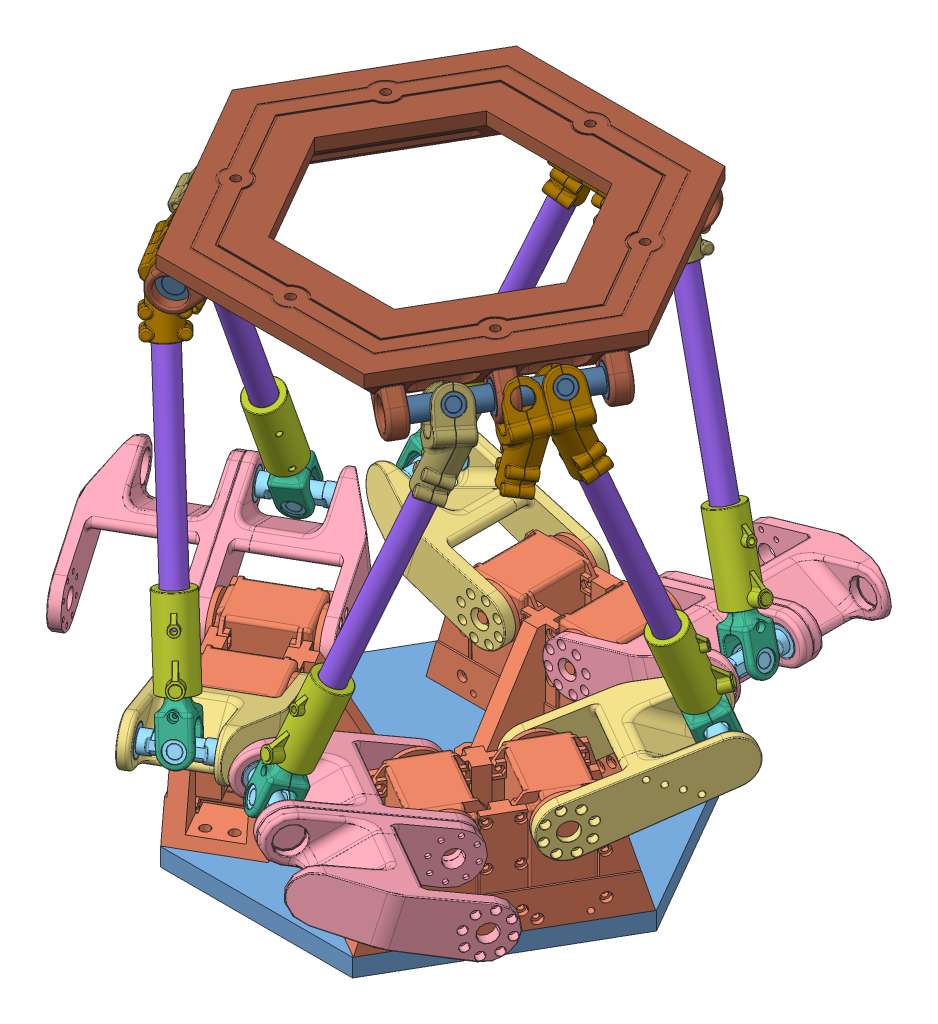
SolidWorks assembly top, configuration Default. Lengths in mm.
Overall size (300.14 294.24 310.35).
47 component instances, 12 part files, 111 mates.
Components (placement in the parent):
- bunn-1: bunn [Default] at origin size (232.33 10 201.21)
- d64hjorne-1: d64hjorne [Default] at (7.8676 41.4552 -80.4625) size (124 64.1 88.1)
- d64hjorne-2: d64hjorne [Default] at (-73.6164 41.4552 33.4177) x (-0.5 0 -0.866025) z (0.866025 0 -0.5) size (124 64.1 88.1)
- d64hjorne-3: d64hjorne [Default] at (65.7488 41.4552 47.0448) x (-0.5 0 0.866025) z (-0.866025 0 -0.5) size (124 64.1 88.1)
- legg-1: legg [Default] at (-73.9624 60.1 70.9924) x (0.477224 0.298375 0.826577) z (0.149187 -0.954449 0.2584) size (96.5 59 29.97)
- leggB-1: leggB [Default] at (85.9279 84.3661 135.8759) x (-0.477224 0.298375 0.826577) z (-0.149187 -0.954449 0.2584) size (96.5 118 29.97)
- kne-1: kne [Default] at (-25.8343 80.9862 120.3528) x (0.177157 -0.935126 0.306845) z (0.467563 0.354314 0.809843) size (15 41.8 16.5)
- laar-1: laar [Default] at (-28.289 79.1261 116.1011) x (-0.836432 -0.119027 0.53499) z (0.285948 -0.92752 0.240707) size (16 18.7 55.01)
- laar2-1: laar2 [Default] at (-32.983 104.1742 114.3351) x (0.61558 0.370312 0.695651) z (-0.734367 -0.050746 0.676853) size (25.4 43 19.2)
- carb-1: carb [Default] at (-38.9879 123.6522 109.2803) x (0.528927 0.362238 0.767476) z (-0.799043 -0.092142 0.594172) size (12 140 12)
- leggB-2: leggB [Default] at (-160.6359 84.3661 6.4779) x (-0.477224 0.298375 -0.826577) z (-0.149187 -0.954449 -0.2584) size (96.5 118 29.97)
- legg-2: legg [Default] at (-24.5 60.1 -99.5495) x (-0.954449 0.298375 0) z (-0.298375 -0.954449 0) size (96.5 59 29.97)
- leggB-3: leggB [Default] at (74.708 84.3661 -142.3537) x (0.954449 0.298375 0) z (0.298375 -0.954449 0) size (96.5 118 29.97)
- legg-4: legg [Default] at (98.4624 60.1 28.5572) x (0.477224 0.298375 -0.826577) z (0.149187 -0.954449 -0.2584) size (96.5 59 29.97)
- kne-2: kne [Default] at (-117.1457 80.9862 -37.8032) x (-0.177157 -0.935126 -0.306845) z (0.467563 -0.354314 0.809843) size (15 41.8 16.5)
- kne-3: kne [Default] at (-91.3114 80.9862 -82.5495) x (-0.354314 -0.935126 0) z (-0.935126 0.354314 0) size (15 41.8 16.5)
- kne-4: kne [Default] at (91.3114 80.9862 -82.5495) x (-0.354314 0.935126 0) z (0.935126 0.354314 0) size (15 41.8 16.5)
- kne-5: kne [Default] at (117.1457 80.9862 -37.8032) x (-0.177157 0.935126 0.306845) z (-0.467563 -0.354314 0.809843) size (15 41.8 16.5)
- kne-6: kne [Default] at (25.8343 80.9862 120.3528) x (0.177157 0.935126 -0.306845) z (-0.467563 0.354314 0.809843) size (15 41.8 16.5)
- laar-2: laar [Default] at (-114.691 79.1261 -33.5516) x (0.881531 0.119027 -0.456876) z (-0.065484 -0.92752 -0.367992) size (16 18.7 55.01)
- laar-3: laar [Default] at (-86.402 79.1261 -82.5495) x (-0.045099 -0.119027 -0.991866) z (-0.351433 -0.92752 0.127285) size (16 18.7 55.01)
- laar-4: laar [Default] at (86.402 79.1261 -82.5495) x (-0.045099 0.119027 0.991866) z (0.351433 -0.92752 0.127285) size (16 18.7 55.01)
- laar-5: laar [Default] at (114.691 79.1261 -33.5516) x (0.881531 -0.119027 0.456876) z (0.065484 -0.92752 -0.367992) size (16 18.7 55.01)
- laar-6: laar [Default] at (28.289 79.1261 116.1011) x (-0.836432 0.119027 -0.53499) z (-0.285948 -0.92752 0.240707) size (16 18.7 55.01)
- laar2-2: laar2 [Default] at (82.5256 104.1742 -85.7317) x (0.935106 0.354369 0.000454) z (-0.045527 0.118865 0.991866) size (25.4 43 19.2)
- laar2-3: laar2 [Default] at (115.5086 104.1742 -28.6034) x (0.719044 0.299561 -0.627087) z (0.691872 -0.223538 0.686545) size (25.4 43 19.2)
- laar2-4: laar2 [Default] at (-82.5256 104.1742 -85.7317) x (-0.874267 0.276499 -0.399006) z (0.334892 -0.251505 -0.908071) size (25.4 43 19.2)
- laar2-5: laar2 [Default] at (-115.5086 104.1742 -28.6034) x (-0.871902 0.232535 -0.430946) z (0.485282 0.292633 -0.823934) size (25.4 43 19.2)
- laar2-6: laar2 [Default] at (32.983 104.1742 114.3351) x (-0.150441 0.291534 0.944656) z (-0.946362 0.23391 -0.222901) size (25.4 43 19.2)
- carb-2: carb [Default] at (-114.1334 123.6522 -20.8756) x (0.997014 -0.075942 0.013991) z (-0.040923 -0.365977 0.929724) size (12 140 12)
- carb-3: carb [Default] at (75.1455 123.6522 -88.4046) x (0.935106 0.354369 0.000454) z (-0.045527 0.118865 0.991866) size (12 140 12)
- carb-4: carb [Default] at (114.1334 123.6522 -20.8756) x (0.995789 0.084455 -0.035668) z (0.064161 -0.364107 0.929145) size (12 140 12)
- carb-5: carb [Default] at (38.9879 123.6522 109.2803) x (0.957578 -0.267218 0.107881) z (-0.035741 0.261344 0.964584) size (12 140 12)
- carb-6: carb [Default] at (-75.1455 123.6522 -88.4046) x (0.009464 0.132431 0.991147) z (-0.936165 0.349526 -0.037763) size (12 140 12)
- topFotGaffel-2: topFotGaffel [Default] at (-98.2015 238.5363 66.8851) x (-0.544987 -0.084611 -0.834164) z (0.726533 -0.544242 -0.419464) size (47.22 50.18 34.26)
- topFotGaffel-3: topFotGaffel [Default] at (-8.8235 238.5363 -118.4875) x (0.994901 -0.084611 -0.05489) z (0 -0.544242 0.838928) size (47.22 50.18 34.26)
- topFotGaffel-4: topFotGaffel [Default] at (107.0249 238.5363 51.6024) x (-0.449914 -0.084611 0.889055) z (-0.726533 -0.544242 -0.419464) size (47.22 50.18 34.26)
- toppKryss-1: toppKryss [Default] at (-23 270.9414 -97.4652) x (0 -0.838928 -0.544242) z (0 -0.544242 0.838928) size (15 44 20)
- toppKryss-2: toppKryss [Default] at (23 270.9414 -97.4652) x (0 0.838928 0.544242) z (0 -0.544242 0.838928) size (15 44 20)
- toppKryss-3: toppKryss [Default] at (-95.9074 270.9414 28.814) x (-0.471327 -0.838928 0.272121) z (0.726533 -0.544242 -0.419464) size (15 44 20)
- toppKryss-4: toppKryss [Default] at (-72.9074 270.9414 68.6512) x (0.471327 0.838928 -0.272121) z (-0.726533 0.544242 0.419464) size (15 44 20)
- toppKryss-5: toppKryss [Default] at (95.9074 270.9414 28.814) x (-0.471327 0.838928 -0.272121) z (0.726533 0.544242 0.419464) size (15 44 20)
- toppKryss-6: toppKryss [Default] at (72.9074 270.9414 68.6512) x (-0.471327 0.838928 -0.272121) z (-0.726533 -0.544242 -0.419464) size (15 44 20)
- topp-1: topp [Default] at (0 264.2404 0) x (0.5 0 0.866025) z (-0.866025 0 0.5) size (237.4 34.3 209.5)
- topFotGaffelB-1: topFotGaffelB [Default] at (-115.1234 240.0593 35.5994) x (-0.449914 0.084611 -0.889055) z (0.726533 -0.544242 -0.419464) size (23.88 50.18 34.26)
- topFotGaffelB-2: topFotGaffelB [Default] at (26.7317 240.0593 -117.4995) x (0.994901 0.084611 0.05489) z (0 -0.544242 0.838928) size (23.88 50.18 34.26)
- topFotGaffelB-3: topFotGaffelB [Default] at (88.3917 240.0593 81.9001) x (-0.544987 0.084611 0.834164) z (-0.726533 -0.544242 -0.419464) size (23.88 50.18 34.26)
Mates (geometry in assembly coordinates):
- Coincident1: coincident anti-aligned: plane of bunn-1 through (0 0 0) normal (0 -1 0)
- Coincident2: coincident aligned: plane of bunn-1 through (0 0 0) normal (0 0 1)
- Coincident3: coincident aligned: plane of bunn-1 through (0 0 0) normal (1 0 0)
- Coincident4: coincident anti-aligned: plane of bunn-1 through (0 10 0) normal (0 1 0); plane of d64hjorne-1 through (62 10 -97.1495) normal (0 -1 0)
- Concentric1: concentric anti-aligned: cylinder of bunn-1 through (0 0 -82.0495) axis (0 1 0) radius 2.45; cylinder of d64hjorne-1 through (0 19 -82.0495) axis (0 -1 0) radius 2.65
- Concentric2: concentric anti-aligned: cylinder of bunn-1 through (0 0 -70.0495) axis (0 1 0) radius 2.45; cylinder of d64hjorne-1 through (0 19 -70.0495) axis (0 -1 0) radius 2.65
- Coincident6: coincident anti-aligned: plane of bunn-1 through (0 10 0) normal (0 1 0); plane of d64hjorne-2 through (-115.134 10 -5.1188) normal (0 -1 0)
- Concentric3: concentric anti-aligned: cylinder of bunn-1 through (-71.057 0 41.0248) axis (0 1 0) radius 2.45; cylinder of d64hjorne-2 through (-71.057 19 41.0248) axis (0 -1 0) radius 2.65
- Concentric4: concentric anti-aligned: cylinder of bunn-1 through (-60.6647 0 35.0248) axis (0 1 0) radius 2.45; cylinder of d64hjorne-2 through (-60.6647 19 35.0248) axis (0 -1 0) radius 2.65
- Coincident7: coincident anti-aligned: plane of bunn-1 through (0 10 0) normal (0 1 0); plane of d64hjorne-3 through (53.134 10 102.2683) normal (0 -1 0)
- Concentric5: concentric anti-aligned: cylinder of bunn-1 through (71.057 0 41.0248) axis (0 1 0) radius 2.45; cylinder of d64hjorne-3 through (71.057 19 41.0248) axis (0 -1 0) radius 2.65
- Concentric6: concentric anti-aligned: cylinder of bunn-1 through (60.6647 0 35.0248) axis (0 1 0) radius 2.45; cylinder of d64hjorne-3 through (60.6647 19 35.0248) axis (0 -1 0) radius 2.65
- Coincident8: coincident anti-aligned: plane of d64hjorne-2 through (-73.9624 60.1 70.9924) normal (-0.866025 0 0.5); plane of legg-1 through (-73.9624 60.1 70.9924) normal (0.866025 0 -0.5)
- Concentric7: concentric aligned: cylinder of d64hjorne-2 through (-76.1275 60.1 72.2424) axis (0.866025 0 -0.5) radius 4.9; cylinder of legg-1 through (-79.1586 60.1 73.9924) axis (0.866025 0 -0.5) radius 5
- Concentric9: concentric anti-aligned: cylinder of legg-1 through (-43.1548 80.9862 130.3528) axis (0.866025 0 -0.5) radius 7.6; cylinder of kne-1 through (-8.6004 80.9862 110.4028) axis (-0.866025 0 0.5) radius 4.9
- Concentric10: concentric aligned: cylinder of kne-1 through (-23.3796 82.8464 124.6045) axis (0.467563 0.354314 0.809843) radius 5.5; cylinder of laar-1 through (-29.6917 78.0631 113.6716) axis (0.467563 0.354314 0.809843) radius 5.6
- Coincident11: coincident aligned: plane of kne-1 through (-28.289 79.1261 116.1011) normal (0.467563 0.354314 0.809843); plane of laar-1 through (-28.289 79.1261 116.1011) normal (0.467563 0.354314 0.809843)
- Coincident12: coincident anti-aligned: plane of d64hjorne-3 through (73.9624 60.1 70.9924) normal (0.866025 0 0.5); plane of leggB-1 through (73.9624 60.1 70.9924) normal (-0.866025 0 -0.5)
- Concentric11: concentric aligned: cylinder of d64hjorne-3 through (29.0374 60.1 45.0549) axis (0.866025 0 0.5) radius 14; cylinder of leggB-1 through (28.0631 60.1 44.4924) axis (0.866025 0 0.5) radius 14
- Concentric12: concentric aligned: cylinder of laar-1 through (-33.8408 106.9568 113.613) axis (0.285948 -0.92752 0.240707) radius 5.4; cylinder of laar2-1 through (-44.4209 141.275 104.7068) axis (0.285948 -0.92752 0.240707) radius 6
- Coincident13: coincident anti-aligned: plane of laar-1 through (-38.702 122.7246 109.521) normal (-0.285948 0.92752 -0.240707); plane of laar2-1 through (-38.702 122.7246 109.521) normal (0.285948 -0.92752 0.240707)
- Concentric13: concentric aligned: cylinder of laar2-1 through (-38.702 122.7246 109.521) axis (0.285948 -0.92752 0.240707) radius 9.6; cylinder of carb-1 through (-79.0207 253.505 75.5813) axis (0.285948 -0.92752 0.240707) radius 6
- Coincident14: coincident anti-aligned: plane of laar2-1 through (-38.9879 123.6522 109.2803) normal (-0.285948 0.92752 -0.240707); plane of carb-1 through (-38.9879 123.6522 109.2803) normal (0.285948 -0.92752 0.240707)
- Concentric14: concentric anti-aligned: cylinder of d64hjorne-2 through (-98.4624 60.1 28.5572) axis (0.866025 0 -0.5) radius 14; cylinder of leggB-2 through (-52.5631 60.1 2.0572) axis (-0.866025 0 0.5) radius 14
- Coincident15: coincident anti-aligned: plane of d64hjorne-2 through (-98.4624 60.1 28.5572) normal (-0.866025 0 0.5); plane of leggB-2 through (-98.4624 60.1 28.5572) normal (0.866025 0 -0.5)
- Concentric15: concentric anti-aligned: cylinder of d64hjorne-1 through (-24.5 60.1 -47.6745) axis (0 0 -1) radius 14; cylinder of legg-2 through (-24.5 60.1 -105.5495) axis (0 0 1) radius 14
- Coincident16: coincident anti-aligned: plane of d64hjorne-1 through (-24.5 60.1 -99.5495) normal (0 0 -1); plane of legg-2 through (-24.5 60.1 -99.5495) normal (0 0 1)
- Concentric17: concentric anti-aligned: cylinder of d64hjorne-1 through (24.5 60.1 -99.5495) axis (0 0 1) radius 14; cylinder of leggB-3 through (24.5 60.1 -46.5495) axis (0 0 -1) radius 14
- Coincident18: coincident anti-aligned: plane of d64hjorne-1 through (24.5 60.1 -99.5495) normal (0 0 -1); plane of leggB-3 through (24.5 60.1 -99.5495) normal (0 0 1)
- Concentric19: concentric aligned: cylinder of d64hjorne-3 through (98.4624 60.1 28.5572) axis (-0.866025 0 -0.5) radius 14; cylinder of legg-4 through (103.6586 60.1 31.5572) axis (-0.866025 0 -0.5) radius 14
- Coincident19: coincident anti-aligned: plane of d64hjorne-3 through (98.4624 60.1 28.5572) normal (0.866025 0 0.5); plane of legg-4 through (98.4624 60.1 28.5572) normal (-0.866025 0 -0.5)
- Width1: width anti-aligned: plane of kne-2 through (-99.4788 80.9862 -48.0032) normal (0.866025 0 -0.5); plane of leggB-2 through (-134.8126 80.9862 -27.6032) normal (-0.866025 0 0.5); plane of kne-2 through (-98.5262 80.9862 -48.5532) normal (-0.866025 0 0.5); plane of leggB-2 through (-135.7653 80.9862 -27.0532) normal (0.866025 0 -0.5)
- Concentric20: concentric anti-aligned: cylinder of leggB-2 through (-56.666 80.9862 -72.7212) axis (-0.866025 0 0.5) radius 12.5; cylinder of kne-2 through (-107.7926 80.9862 -43.2032) axis (0.866025 0 -0.5) radius 5.4
- Concentric21: concentric anti-aligned: cylinder of legg-2 through (-91.3114 80.9862 -12.7136) axis (0 0 -1) radius 12.5; cylinder of kne-3 through (-91.3114 80.9862 -71.7495) axis (0 0 1) radius 5.4
- Width2: width anti-aligned: plane of kne-3 through (-91.3114 80.9862 -102.9495) normal (0 0 -1); plane of legg-2 through (-91.3114 80.9862 -62.1495) normal (0 0 1); plane of kne-3 through (-91.3114 80.9862 -104.0495) normal (0 0 1); plane of legg-2 through (-91.3114 80.9862 -61.0495) normal (0 0 -1)
- Concentric22: concentric anti-aligned: cylinder of leggB-3 through (91.3114 80.9862 -59.5495) axis (0 0 -1) radius 12.5; cylinder of kne-4 through (91.3114 80.9862 -71.7495) axis (0 0 1) radius 5.4
- Width3: width anti-aligned: plane of leggB-3 through (91.3114 80.9862 -61.0495) normal (0 0 -1); plane of kne-4 through (91.3114 80.9862 -104.0495) normal (0 0 1); plane of leggB-3 through (91.3114 80.9862 -62.1495) normal (0 0 1); plane of kne-4 through (91.3114 80.9862 -102.9495) normal (0 0 -1)
- Concentric23: concentric anti-aligned: cylinder of legg-4 through (56.666 80.9862 -72.7212) axis (0.866025 0 0.5) radius 12.5; cylinder of kne-5 through (107.7926 80.9862 -43.2032) axis (-0.866025 0 -0.5) radius 5.4
- Width4: width anti-aligned: plane of kne-5 through (99.4788 80.9862 -48.0032) normal (-0.866025 0 -0.5); plane of legg-4 through (134.8126 80.9862 -27.6032) normal (0.866025 0 0.5); plane of kne-5 through (98.5262 80.9862 -48.5532) normal (0.866025 0 0.5); plane of legg-4 through (135.7653 80.9862 -27.0532) normal (-0.866025 0 -0.5)
- Concentric24: concentric anti-aligned: cylinder of leggB-1 through (-34.6454 80.9862 85.4348) axis (0.866025 0 0.5) radius 12.5; cylinder of kne-6 through (16.4812 80.9862 114.9528) axis (-0.866025 0 -0.5) radius 5.4
- Width5: width anti-aligned: plane of leggB-1 through (7.2147 80.9862 109.6028) normal (0.866025 0 0.5); plane of kne-6 through (44.4538 80.9862 131.1028) normal (-0.866025 0 -0.5); plane of leggB-1 through (8.1674 80.9862 110.1528) normal (-0.866025 0 -0.5); plane of kne-6 through (43.5012 80.9862 130.5528) normal (0.866025 0 0.5)
- Width6: width anti-aligned: plane of kne-1 through (-43.5012 80.9862 130.5528) normal (-0.866025 0 0.5); plane of legg-1 through (-8.1674 80.9862 110.1528) normal (0.866025 0 -0.5); plane of kne-1 through (-44.4538 80.9862 131.1028) normal (0.866025 0 -0.5); plane of legg-1 through (-7.2147 80.9862 109.6028) normal (-0.866025 0 0.5)
- Concentric25: concentric anti-aligned: cylinder of kne-6 through (21.9769 83.9093 127.034) axis (0.467563 -0.354314 -0.809843) radius 3.4; cylinder of laar-6 through (29.6917 78.0631 113.6716) axis (-0.467563 0.354314 0.809843) radius 5.6
- Width7: width aligned: plane of laar-6 through (21.4626 84.2991 127.9248) normal (-0.467563 0.354314 0.809843); plane of kne-6 through (30.206 77.6734 112.7807) normal (0.467563 -0.354314 -0.809843); plane of laar-6 through (21.9769 83.9093 127.034) normal (-0.467563 0.354314 0.809843); plane of kne-6 through (29.6917 78.0631 113.6716) normal (0.467563 -0.354314 -0.809843)
- Concentric26: concentric aligned: cylinder of kne-5 through (113.2883 78.0631 -31.122) axis (0.467563 0.354314 -0.809843) radius 3.4; cylinder of laar-5 through (113.2883 78.0631 -31.122) axis (0.467563 0.354314 -0.809843) radius 5.6
- Width8: width anti-aligned: plane of laar-5 through (112.774 77.6734 -30.2312) normal (-0.467563 -0.354314 0.809843); plane of kne-5 through (121.5174 84.2991 -45.3753) normal (0.467563 0.354314 -0.809843); plane of laar-5 through (121.0031 83.9093 -44.4844) normal (0.467563 0.354314 -0.809843); plane of kne-5 through (113.2883 78.0631 -31.122) normal (-0.467563 -0.354314 0.809843)
- Concentric27: concentric anti-aligned: cylinder of kne-4 through (99.0262 83.9093 -82.5495) axis (-0.935126 -0.354314 0) radius 3.4; cylinder of laar-4 through (83.5966 78.0631 -82.5495) axis (0.935126 0.354314 0) radius 5.6
- Width9: width anti-aligned: plane of laar-4 through (82.568 77.6734 -82.5495) normal (-0.935126 -0.354314 0); plane of kne-4 through (100.0549 84.2991 -82.5495) normal (0.935126 0.354314 0); plane of laar-4 through (99.0262 83.9093 -82.5495) normal (0.935126 0.354314 0); plane of kne-4 through (83.5966 78.0631 -82.5495) normal (-0.935126 -0.354314 0)
- Concentric28: concentric aligned: cylinder of kne-2 through (-113.2883 78.0631 -31.122) axis (-0.467563 0.354314 -0.809843) radius 3.4; cylinder of laar-2 through (-113.2883 78.0631 -31.122) axis (-0.467563 0.354314 -0.809843) radius 5.6
- Width10: width anti-aligned: plane of laar-2 through (-121.5174 84.2991 -45.3753) normal (-0.467563 0.354314 -0.809843); plane of kne-2 through (-112.774 77.6734 -30.2312) normal (0.467563 -0.354314 0.809843); plane of laar-2 through (-113.2883 78.0631 -31.122) normal (0.467563 -0.354314 0.809843); plane of kne-2 through (-121.0031 83.9093 -44.4844) normal (-0.467563 0.354314 -0.809843)
- Concentric29: concentric anti-aligned: cylinder of kne-3 through (-99.0262 83.9093 -82.5495) axis (0.935126 -0.354314 0) radius 3.4; cylinder of laar-3 through (-83.5966 78.0631 -82.5495) axis (-0.935126 0.354314 0) radius 5.6
- Width11: width anti-aligned: plane of laar-3 through (-82.568 77.6734 -82.5495) normal (0.935126 -0.354314 0); plane of kne-3 through (-100.0549 84.2991 -82.5495) normal (-0.935126 0.354314 0); plane of laar-3 through (-99.0262 83.9093 -82.5495) normal (-0.935126 0.354314 0); plane of kne-3 through (-83.5966 78.0631 -82.5495) normal (0.935126 -0.354314 0)
- Coincident20: coincident anti-aligned: plane of laar-6 through (38.702 122.7246 109.521) normal (0.285948 0.92752 -0.240707); plane of laar2-6 through (38.702 122.7246 109.521) normal (-0.285948 -0.92752 0.240707)
- Concentric30: concentric aligned: cylinder of laar-6 through (34.9846 110.6669 112.6502) axis (-0.285948 -0.92752 0.240707) radius 7.5; cylinder of laar2-6 through (38.702 122.7246 109.521) axis (-0.285948 -0.92752 0.240707) radius 9.6
- Coincident21: coincident anti-aligned: plane of laar-5 through (114.1989 122.7246 -21.2436) normal (-0.065484 0.92752 0.367992); plane of laar2-3 through (114.1989 122.7246 -21.2436) normal (0.065484 -0.92752 -0.367992)
- Concentric31: concentric anti-aligned: cylinder of laar-5 through (114.4609 119.0146 -22.7156) axis (-0.065484 0.92752 0.367992) radius 7.5; cylinder of laar2-3 through (114.1989 122.7246 -21.2436) axis (0.065484 -0.92752 -0.367992) radius 9.6
- Coincident22: coincident anti-aligned: plane of laar-4 through (75.497 122.7246 -88.2774) normal (-0.351433 0.92752 -0.127285); plane of laar2-2 through (75.497 122.7246 -88.2774) normal (0.351433 -0.92752 0.127285)
- Concentric32: concentric anti-aligned: cylinder of laar-4 through (76.9027 119.0146 -87.7682) axis (-0.351433 0.92752 -0.127285) radius 7.5; cylinder of laar2-2 through (75.497 122.7246 -88.2774) axis (0.351433 -0.92752 0.127285) radius 9.6
- Coincident23: coincident anti-aligned: plane of laar-3 through (-75.497 122.7246 -88.2774) normal (0.351433 0.92752 -0.127285); plane of laar2-4 through (-75.497 122.7246 -88.2774) normal (-0.351433 -0.92752 0.127285)
- Concentric33: concentric anti-aligned: cylinder of laar-3 through (-76.9027 119.0146 -87.7682) axis (0.351433 0.92752 -0.127285) radius 7.5; cylinder of laar2-4 through (-75.497 122.7246 -88.2774) axis (-0.351433 -0.92752 0.127285) radius 9.6
- Coincident24: coincident anti-aligned: plane of laar-2 through (-114.1989 122.7246 -21.2436) normal (0.065484 0.92752 0.367992); plane of laar2-5 through (-114.1989 122.7246 -21.2436) normal (-0.065484 -0.92752 -0.367992)
- Concentric34: concentric anti-aligned: cylinder of laar-2 through (-114.4609 119.0146 -22.7156) axis (0.065484 0.92752 0.367992) radius 7.5; cylinder of laar2-5 through (-114.1989 122.7246 -21.2436) axis (-0.065484 -0.92752 -0.367992) radius 9.6
- Coincident25: coincident anti-aligned: plane of laar2-4 through (-75.1455 123.6522 -88.4046) normal (0.351433 0.92752 -0.127285); plane of carb-6 through (-75.1455 123.6522 -88.4046) normal (-0.351433 -0.92752 0.127285)
- Concentric35: concentric aligned: cylinder of laar2-4 through (-75.497 122.7246 -88.2774) axis (-0.351433 -0.92752 0.127285) radius 9.6; cylinder of carb-6 through (-25.945 253.505 -106.2245) axis (-0.351433 -0.92752 0.127285) radius 6
- Coincident26: coincident anti-aligned: plane of laar2-2 through (75.1455 123.6522 -88.4046) normal (-0.351433 0.92752 -0.127285); plane of carb-3 through (75.1455 123.6522 -88.4046) normal (0.351433 -0.92752 0.127285)
- Concentric36: concentric aligned: cylinder of laar2-2 through (75.497 122.7246 -88.2774) axis (0.351433 -0.92752 0.127285) radius 9.6; cylinder of carb-3 through (25.945 253.505 -106.2245) axis (0.351433 -0.92752 0.127285) radius 6
- Coincident27: coincident anti-aligned: plane of laar2-5 through (-114.1334 123.6522 -20.8756) normal (0.065484 0.92752 0.367992); plane of carb-2 through (-114.1334 123.6522 -20.8756) normal (-0.065484 -0.92752 -0.367992)
- Concentric37: concentric aligned: cylinder of laar2-5 through (-114.1989 122.7246 -21.2436) axis (-0.065484 -0.92752 -0.367992) radius 9.6; cylinder of carb-2 through (-104.9656 253.505 30.6433) axis (-0.065484 -0.92752 -0.367992) radius 6
- Coincident28: coincident anti-aligned: plane of laar2-6 through (38.9879 123.6522 109.2803) normal (0.285948 0.92752 -0.240707); plane of carb-5 through (38.9879 123.6522 109.2803) normal (-0.285948 -0.92752 0.240707)
- Concentric38: concentric aligned: cylinder of laar2-6 through (38.702 122.7246 109.521) axis (-0.285948 -0.92752 0.240707) radius 9.6; cylinder of carb-5 through (79.0207 253.505 75.5813) axis (-0.285948 -0.92752 0.240707) radius 6
- Coincident29: coincident anti-aligned: plane of laar2-3 through (114.1334 123.6522 -20.8756) normal (-0.065484 0.92752 0.367992); plane of carb-4 through (114.1334 123.6522 -20.8756) normal (0.065484 -0.92752 -0.367992)
- Concentric39: concentric aligned: cylinder of laar2-3 through (114.1989 122.7246 -21.2436) axis (0.065484 -0.92752 -0.367992) radius 9.6; cylinder of carb-4 through (104.9656 253.505 30.6433) axis (0.065484 -0.92752 -0.367992) radius 6
- Parallel8: parallel aligned: plane of bunn-1 through (0 10 0) normal (0 1 0); plane of topp-1 through (0 294.2404 0) normal (0 1 0)
- Concentric52: concentric aligned: cylinder of toppKryss-5 through (84.9074 270.9414 47.8666) axis (0.5 0 -0.866025) radius 4.9; cylinder of topp-1 through (90.9074 270.9414 37.4743) axis (0.5 0 -0.866025) radius 7.6
- Concentric53: concentric aligned: cylinder of toppKryss-6 through (83.9074 270.9414 49.5986) axis (-0.5 0 0.866025) radius 4.9; cylinder of topp-1 through (77.9074 270.9414 59.9909) axis (-0.5 0 0.866025) radius 7.6
- Width15: width anti-aligned: plane of toppKryss-5 through (106.9074 270.9414 9.7615) normal (0.5 0 -0.866025); plane of topp-1 through (84.9074 270.9414 47.8666) normal (-0.5 0 0.866025); plane of toppKryss-5 through (89.5981 273.0627 4.3867) normal (-0.5 0 0.866025); plane of topp-1 through (71.5981 273.0627 35.5637) normal (0.5 0 -0.866025)
- Width16: width anti-aligned: plane of toppKryss-6 through (61.9074 270.9414 87.7038) normal (-0.5 0 0.866025); plane of topp-1 through (83.9074 270.9414 49.5986) normal (0.5 0 -0.866025); plane of toppKryss-6 through (48.5981 273.0627 75.4008) normal (0.5 0 -0.866025); plane of topp-1 through (66.5981 273.0627 44.2239) normal (-0.5 0 0.866025)
- Concentric54: concentric aligned: cylinder of toppKryss-2 through (1 270.9414 -97.4652) axis (1 0 0) radius 4.9; cylinder of topp-1 through (13 270.9414 -97.4652) axis (1 0 0) radius 7.6
- Concentric55: concentric aligned: cylinder of toppKryss-1 through (-1 270.9414 -97.4652) axis (-1 0 0) radius 4.9; cylinder of topp-1 through (-13 270.9414 -97.4652) axis (-1 0 0) radius 7.6
- Concentric56: concentric anti-aligned: cylinder of toppKryss-3 through (-106.9074 270.9414 9.7615) axis (0.5 0 0.866025) radius 4.9; cylinder of topp-1 through (-90.9074 270.9414 37.4743) axis (-0.5 0 -0.866025) radius 7.6
- Concentric57: concentric aligned: cylinder of toppKryss-4 through (-83.9074 270.9414 49.5986) axis (0.5 0 0.866025) radius 4.9; cylinder of topp-1 through (-100.9074 270.9414 20.1538) axis (0.5 0 0.866025) radius 7.6
- Width17: width anti-aligned: plane of toppKryss-3 through (-106.9074 270.9414 9.7615) normal (-0.5 0 -0.866025); plane of topp-1 through (-84.9074 270.9414 47.8666) normal (0.5 0 0.866025); plane of toppKryss-3 through (-89.5981 273.0627 4.3867) normal (0.5 0 0.866025); plane of topp-1 through (-71.5981 273.0627 35.5637) normal (-0.5 0 -0.866025)
- Width18: width anti-aligned: plane of toppKryss-4 through (-83.9074 270.9414 49.5986) normal (-0.5 0 -0.866025); plane of topp-1 through (-61.9074 270.9414 87.7038) normal (0.5 0 0.866025); plane of toppKryss-4 through (-66.5981 273.0627 44.2239) normal (0.5 0 0.866025); plane of topp-1 through (-48.5981 273.0627 75.4008) normal (-0.5 0 -0.866025)
- Width19: width anti-aligned: plane of toppKryss-1 through (-45 270.9414 -97.4652) normal (-1 0 0); plane of topp-1 through (-1 270.9414 -97.4652) normal (1 0 0); plane of toppKryss-1 through (-41 273.0627 -79.7876) normal (1 0 0); plane of topp-1 through (-5 273.0627 -79.7876) normal (-1 0 0)
- Width20: width anti-aligned: plane of toppKryss-2 through (1 270.9414 -97.4652) normal (-1 0 0); plane of topp-1 through (45 270.9414 -97.4652) normal (1 0 0); plane of toppKryss-2 through (5 273.0627 -79.7876) normal (1 0 0); plane of topp-1 through (41 273.0627 -79.7876) normal (-1 0 0)
- Coincident30: coincident aligned: line of topp-1 through (0 295.9053 0) axis (0 -1 0)
- Coincident31: coincident anti-aligned: plane of carb-1 through (-79.0207 253.505 75.5813) normal (-0.285948 0.92752 -0.240707); plane of topFotGaffel-2 through (-79.0207 253.505 75.5813) normal (0.285948 -0.92752 0.240707)
- Concentric59: concentric anti-aligned: cylinder of carb-1 through (-79.0207 253.505 75.5813) axis (0.285948 -0.92752 0.240707) radius 6; cylinder of topFotGaffel-2 through (-73.3017 234.9546 80.3954) axis (-0.285948 0.92752 -0.240707) radius 8.075
- Concentric62: concentric aligned: cylinder of topFotGaffel-2 through (-62.0094 262.7778 62.3592) axis (-0.726533 0.544242 0.419464) radius 5.6; cylinder of toppKryss-4 through (-77.9931 274.7511 71.5874) axis (-0.726533 0.544242 0.419464) radius 5.5
- Width21: width aligned: plane of topFotGaffel-2 through (-91.2446 265.3161 70.4128) normal (-0.726533 0.544242 0.419464); plane of toppKryss-4 through (-75.2608 253.3428 61.1846) normal (0.726533 -0.544242 -0.419464); plane of topFotGaffel-2 through (-80.1727 276.3838 72.8458) normal (-0.726533 0.544242 0.419464); plane of toppKryss-4 through (-65.642 265.499 64.4566) normal (0.726533 -0.544242 -0.419464)
- Parallel10: parallel aligned: plane of bunn-1 through (-170 10 -98.1495) normal (-0.866025 0 0.5); plane of topp-1 through (-175 294.2404 -101.0363) normal (-0.866025 0 0.5)
- Concentric63: concentric aligned: cylinder of topFotGaffel-3 through (-23 262.7778 -84.8813) axis (0 0.544242 -0.838928) radius 5.6; cylinder of toppKryss-1 through (-23 274.7511 -103.3377) axis (0 0.544242 -0.838928) radius 5.5
- Width22: width aligned: plane of topFotGaffel-3 through (-15.357 265.3161 -114.2265) normal (0 0.544242 -0.838928); plane of topFotGaffel-3 through (-15.357 253.3428 -95.7701) normal (0 -0.544242 0.838928); plane of toppKryss-1 through (-23 276.3838 -105.8545) normal (0 0.544242 -0.838928); plane of toppKryss-1 through (-23 265.499 -89.0759) normal (0 -0.544242 0.838928)
- Concentric64: concentric anti-aligned: cylinder of carb-6 through (-25.945 253.505 -106.2245) axis (-0.351433 -0.92752 0.127285) radius 6; cylinder of topFotGaffel-3 through (-32.9736 234.9546 -103.6788) axis (0.351433 0.92752 -0.127285) radius 8.075
- Coincident32: coincident anti-aligned: plane of carb-6 through (-25.945 253.505 -106.2245) normal (0.351433 0.92752 -0.127285); plane of topFotGaffel-3 through (-25.945 253.505 -106.2245) normal (-0.351433 -0.92752 0.127285)
- Concentric65: concentric aligned: cylinder of topFotGaffel-4 through (85.0094 262.7778 22.5221) axis (0.726533 0.544242 0.419464) radius 5.6; cylinder of toppKryss-5 through (100.9931 274.7511 31.7503) axis (0.726533 0.544242 0.419464) radius 5.5
- Width23: width anti-aligned: plane of topFotGaffel-4 through (106.6016 265.3161 43.8137) normal (0.726533 0.544242 0.419464); plane of topFotGaffel-4 through (90.6178 253.3428 34.5855) normal (-0.726533 -0.544242 -0.419464); plane of toppKryss-5 through (88.642 265.499 24.6194) normal (-0.726533 -0.544242 -0.419464); plane of toppKryss-5 through (103.1727 276.3838 33.0087) normal (0.726533 0.544242 0.419464)
- Concentric66: concentric anti-aligned: cylinder of carb-4 through (104.9656 253.505 30.6433) axis (0.065484 -0.92752 -0.367992) radius 6; cylinder of topFotGaffel-4 through (106.2753 234.9546 23.2834) axis (-0.065484 0.92752 0.367992) radius 8.075
- Coincident33: coincident anti-aligned: plane of carb-4 through (104.9656 253.505 30.6433) normal (-0.065484 0.92752 0.367992); plane of topFotGaffel-4 through (104.9656 253.505 30.6433) normal (0.065484 -0.92752 -0.367992)
- Concentric67: concentric aligned: cylinder of toppKryss-3 through (-100.9931 274.7511 31.7503) axis (-0.726533 0.544242 0.419464) radius 5.5; cylinder of topFotGaffelB-1 through (-85.0094 262.7778 22.5221) axis (-0.726533 0.544242 0.419464) radius 5.6
- Width24: width anti-aligned: plane of topFotGaffelB-1 through (-106.6016 265.3161 43.8137) normal (-0.726533 0.544242 0.419464); plane of topFotGaffelB-1 through (-90.6178 253.3428 34.5855) normal (0.726533 -0.544242 -0.419464); plane of toppKryss-3 through (-88.642 265.499 24.6194) normal (0.726533 -0.544242 -0.419464); plane of toppKryss-3 through (-103.1727 276.3838 33.0087) normal (-0.726533 0.544242 0.419464)
- Concentric68: concentric anti-aligned: cylinder of carb-2 through (-104.9656 253.505 30.6433) axis (-0.065484 -0.92752 -0.367992) radius 6; cylinder of topFotGaffelB-1 through (-106.2753 234.9546 23.2834) axis (0.065484 0.92752 0.367992) radius 8.075
- Coincident34: coincident anti-aligned: plane of carb-2 through (-104.9656 253.505 30.6433) normal (0.065484 0.92752 0.367992); plane of topFotGaffelB-1 through (-104.9656 253.505 30.6433) normal (-0.065484 -0.92752 -0.367992)
- Concentric69: concentric aligned: cylinder of toppKryss-2 through (23 274.7511 -103.3377) axis (0 0.544242 -0.838928) radius 5.5; cylinder of topFotGaffelB-2 through (23 262.7778 -84.8813) axis (0 0.544242 -0.838928) radius 5.6
- Width25: width anti-aligned: plane of topFotGaffelB-2 through (15.357 265.3161 -114.2265) normal (0 0.544242 -0.838928); plane of topFotGaffelB-2 through (15.357 253.3428 -95.7701) normal (0 -0.544242 0.838928); plane of toppKryss-2 through (23 265.499 -89.0759) normal (0 -0.544242 0.838928); plane of toppKryss-2 through (23 276.3838 -105.8545) normal (0 0.544242 -0.838928)
- Concentric70: concentric anti-aligned: cylinder of carb-3 through (25.945 253.505 -106.2245) axis (0.351433 -0.92752 0.127285) radius 6; cylinder of topFotGaffelB-2 through (32.9736 234.9546 -103.6788) axis (-0.351433 0.92752 -0.127285) radius 8.075
- Coincident35: coincident anti-aligned: plane of carb-3 through (25.945 253.505 -106.2245) normal (-0.351433 0.92752 -0.127285); plane of topFotGaffelB-2 through (25.945 253.505 -106.2245) normal (0.351433 -0.92752 0.127285)
- Concentric71: concentric aligned: cylinder of toppKryss-6 through (77.9931 274.7511 71.5874) axis (0.726533 0.544242 0.419464) radius 5.5; cylinder of topFotGaffelB-3 through (62.0094 262.7778 62.3592) axis (0.726533 0.544242 0.419464) radius 5.6
- Width26: width anti-aligned: plane of topFotGaffelB-3 through (91.2446 265.3161 70.4128) normal (0.726533 0.544242 0.419464); plane of topFotGaffelB-3 through (75.2608 253.3428 61.1846) normal (-0.726533 -0.544242 -0.419464); plane of toppKryss-6 through (80.1727 276.3838 72.8458) normal (0.726533 0.544242 0.419464); plane of toppKryss-6 through (65.642 265.499 64.4566) normal (-0.726533 -0.544242 -0.419464)
- Concentric72: concentric anti-aligned: cylinder of carb-5 through (79.0207 253.505 75.5813) axis (-0.285948 -0.92752 0.240707) radius 6; cylinder of topFotGaffelB-3 through (73.3017 234.9546 80.3954) axis (0.285948 0.92752 -0.240707) radius 8.075
- Coincident36: coincident anti-aligned: plane of carb-5 through (79.0207 253.505 75.5813) normal (0.285948 0.92752 -0.240707); plane of topFotGaffelB-3 through (79.0207 253.505 75.5813) normal (-0.285948 -0.92752 0.240707)
